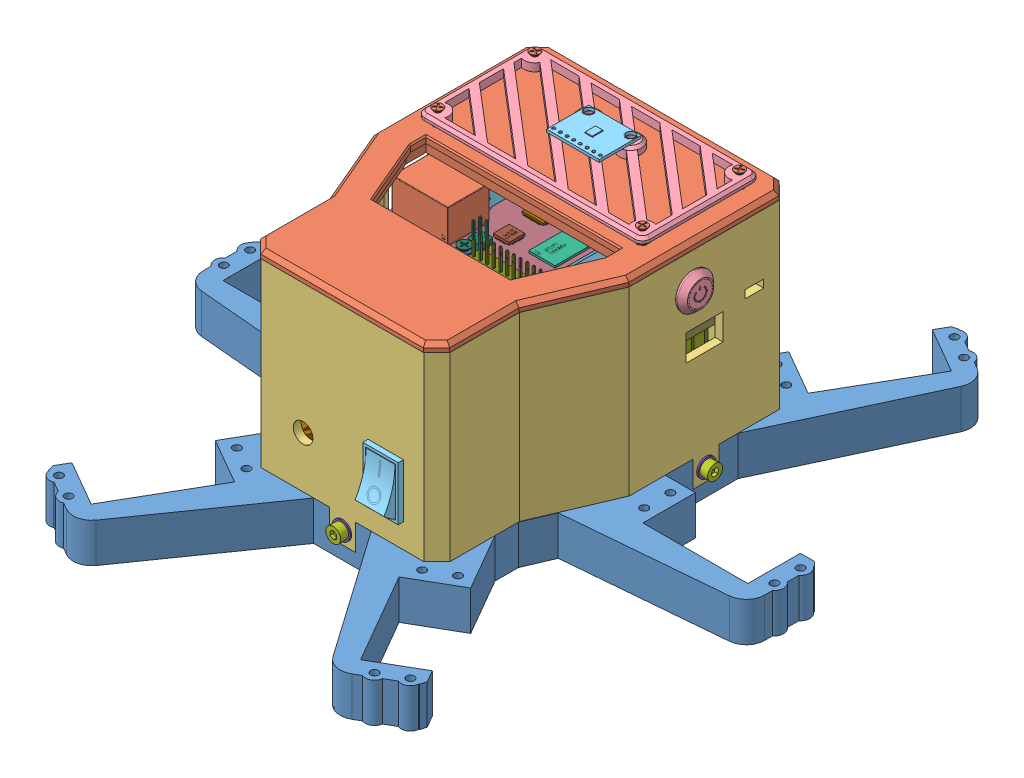
SolidWorks assembly BODY_ASM, configuration Default. Lengths in mm.
Overall size (216.8 93.6 230.48).
146 component instances, 41 part files, 76 mates.
Components (placement in the parent):
- MAIN_FRAME-1: MAIN_FRAME [Default] at origin size (216.8 15 230.48)
- LID-1: LID [Default] at (-25.1298 69 304.4932) x (1 0 0) z (0 1 0) size (97 123 7)
- MID CASE-1: MID CASE [Default] at origin size (97 79 123)
- ON_SWITCH-1: ON_SWITCH [Default] at (33.5 56 5) x (0 0.109318 -0.994007) z (0 -0.994007 -0.109318) size (13.7 18.1 13.7)
- POWER_SWITCH-1: POWER_SWITCH [Default] at (16.5 19.5 76) x (0 -1 0) z (-1 0 0) size (20.5 20.17 13.5)
- M3_HEX_NUT-1: M3_HEX_NUT [Default] at (-35 -5 0) x (0 -0.865861 0.500284) z (0 0.500284 0.865861) size (6.98 2.4 5.5)
- M3_STEEL_HEX_BOLT_16MM-1: M3_STEEL_HEX_BOLT_16MM [Default] at (0 -5 -36.5) x (0.06898 0.997618 0) z (0.997618 -0.06898 0) size (5.68 19 5.68)
- M3_WASHER-1: M3_WASHER [Default] at (-49 -5 0) x (0 -0.533756 -0.845639) z (0 -0.845639 0.533756) size (7 0.5 7)
- M3_HEX_NUT-2: M3_HEX_NUT [Default] at (0 -5 -20.5) x (0.938223 0.346031 0) z (0.346031 -0.938223 0) size (6.98 2.4 5.5)
- M3_HEX_NUT-3: M3_HEX_NUT [Default] at (0 -5 75.1) x (0.997389 -0.072217 0) z (-0.072217 -0.997389 0) size (6.98 2.4 5.5)
- M3_HEX_NUT-4: M3_HEX_NUT [Default] at (32.6 -5 0) x (0 -0.520946 -0.85359) z (0 -0.85359 0.520946) size (6.98 2.4 5.5)
- M3_STEEL_HEX_BOLT_16MM-2: M3_STEEL_HEX_BOLT_16MM [Default] at (-52 -5 0) x (0 -0.536208 -0.844086) z (0 -0.844086 0.536208) size (5.68 19 5.68)
- M3_STEEL_HEX_BOLT_16MM-3: M3_STEEL_HEX_BOLT_16MM [Default] at (52 -5 0) x (0 0.249062 -0.968488) z (0 0.968488 0.249062) size (5.68 19 5.68)
- M3_STEEL_HEX_BOLT_16MM-4: M3_STEEL_HEX_BOLT_16MM [Default] at (0 -5 93.5) x (-0.010084 0.999949 0) z (-0.999949 -0.010084 0) size (5.68 19 5.68)
- M3_WASHER-2: M3_WASHER [Default] at (48.5 -5 0) x (0 -0.753455 -0.657499) z (0 -0.657499 0.753455) size (7 0.5 7)
- M3_WASHER-3: M3_WASHER [Default] at (0 -5 90.5) x (0.583401 0.812184 0) z (-0.812184 0.583401 0) size (7 0.5 7)
- M3_WASHER-4: M3_WASHER [Default] at (0 -5 -33) x (0.7999 0.600134 0) z (-0.600134 0.7999 0) size (7 0.5 7)
- INNER_FRAME_ASM_BRASS-1: INNER_FRAME_ASM_BRASS [Default] at (0 3.6 0) size (89.3 62.14 116.59)
  - power frame R-1: power frame R [Default] at origin size (85 4 113)
  - M2.5_STEEL_HEX_NUT-1: M2.5_STEEL_HEX_NUT [Default] at (39 -1.8 -24.5) x (-0.53176 0 -0.846895) z (0.846895 0 -0.53176) size (6.22 1.8 4.9)
  - M2.5_STEEL_HEX_NUT-2: M2.5_STEEL_HEX_NUT [Default] at (-28.3 -1.8 82.3) x (-0.926596 0 0.376059) z (-0.376059 0 -0.926596) size (6.22 1.8 4.9)
  - M2.5_STEEL_HEX_NUT-3: M2.5_STEEL_HEX_NUT [Default] at (28.3 -1.8 82.3) x (-0.90596 0 -0.423363) z (0.423363 0 -0.90596) size (6.22 1.8 4.9)
  - M2.5_STEEL_HEX_NUT-4: M2.5_STEEL_HEX_NUT [Default] at (-19 -1.8 -24.5) x (0.987479 0 -0.157753) z (0.157753 0 0.987479) size (6.22 1.8 4.9)
  - M2.5_BRASS_SPACER_20MM-1: M2.5_BRASS_SPACER_20MM [Default] at (28.3 16.5 82.3) x (0.147579 0 -0.98905) z (0.98905 0 0.147579) size (5.43 25 4.7)
  - M2.5_BRASS_SPACER_20MM-2: M2.5_BRASS_SPACER_20MM [Default] at (-19 16.5 -24.5) x (0.999419 0 0.034097) z (-0.034097 0 0.999419) size (5.43 25 4.7)
  - M2.5_BRASS_SPACER_20MM-3: M2.5_BRASS_SPACER_20MM [Default] at (-28.3 16.5 82.3) x (0.586169 0 0.810189) z (-0.810189 0 0.586169) size (5.43 25 4.7)
  - M2.5_BRASS_SPACER_20MM-4: M2.5_BRASS_SPACER_20MM [Default] at (39 16.5 -24.5) x (0.00416 0 -0.999991) z (0.999991 0 0.00416) size (5.43 25 4.7)
  - RPi FRAME-1: RPi FRAME [Default] at (0 30.8 0) size (85 4 113)
  - M2.5_STEEL_HEX_NUT-9: M2.5_STEEL_HEX_NUT [Default] at (39 34.8 -24.5) x (0.941663 0 -0.336557) z (0.336557 0 0.941663) size (6.22 1.8 4.9)
  - M2.5_STEEL_HEX_NUT-10: M2.5_STEEL_HEX_NUT [Default] at (28.3 34.8 82.3) x (-0.299428 0 -0.954119) z (0.954119 0 -0.299428) size (6.22 1.8 4.9)
  - M2.5_STEEL_HEX_NUT-11: M2.5_STEEL_HEX_NUT [Default] at (28.3 34.8 45.7) x (-0.609973 0 0.792422) z (-0.792422 0 -0.609973) size (6.22 1.8 4.9)
  - M2.5_STEEL_HEX_NUT-12: M2.5_STEEL_HEX_NUT [Default] at (39 34.8 24.5) x (-0.398443 0 0.917193) z (-0.917193 0 -0.398443) size (6.22 1.8 4.9)
  - M2.5_STEEL_HEX_NUT-13: M2.5_STEEL_HEX_NUT [Default] at (-19 34.8 -24.5) x (-0.889727 0 0.456493) z (-0.456493 0 -0.889727) size (6.22 1.8 4.9)
  - M2.5_STEEL_HEX_NUT-14: M2.5_STEEL_HEX_NUT [Default] at (-19 34.8 24.5) x (-0.550521 0 -0.834821) z (0.834821 0 -0.550521) size (6.22 1.8 4.9)
  - M2.5_STEEL_HEX_NUT-15: M2.5_STEEL_HEX_NUT [Default] at (-28.3 34.8 82.3) x (-0.427939 0 0.903808) z (-0.903808 0 -0.427939) size (6.22 1.8 4.9)
  - M2.5_STEEL_HEX_NUT-16: M2.5_STEEL_HEX_NUT [Default] at (-28.3 34.8 45.7) x (-0.613101 0 -0.790005) z (0.790005 0 -0.613101) size (6.22 1.8 4.9)
  - Raspberry Pi 4 Model B-1: Raspberry Pi 4 Model B [Default] at (0 39.19 0) x (-1 0 0) z (0 0 -1) size (88.99 19.9 58.4)
    - PCB, RPi4ModelB-1: PCB, RPi4ModelB [Default] at origin size (85 1.6 56)
    - Broadcom BCM2711B0 CPU, RPi4ModelB-1: Broadcom BCM2711B0 CPU, RPi4ModelB [Default] at (-13.25 0.8 -4.5) size (15 2.3 15)
    - 2.54 mm DUPONT MALE PIN HEADER, POE, 2X2, RPi4ModelB-1: 2.54 mm DUPONT MALE PIN HEADER, POE, 2X2, RPi4ModelB [Default] at (19 0.8 -18.5) size (5.08 11.3 5.08)
    - 2.54 mm DUPONT MALE PIN HEADER, IO, 2X20, RPi4ModelB-1: 2.54 mm DUPONT MALE PIN HEADER, IO, 2X20, RPi4ModelB [Default] at (-10 0.8 -24.5) size (50.8 11.3 5.08)
    - Camera Connector, RPi4ModelB-1: Camera Connector, RPi4ModelB [Default] at (4 0.8 16.5) x (0 0 -1) z (1 0 0) size (22.4 5.68 5.07)
    - Microphone Plug, RPi4ModelB-1: Microphone Plug, RPi4ModelB [Default] at (11.5 0.8 21.65) size (7.23 7.55 15)
    - Display Connector, RPi4ModelB-1: Display Connector, RPi4ModelB [Default] at (-38.5 0.8 0) x (0 0 1) z (-1 0 0) size (22.4 5.68 5.07)
    - Gigabit Ethernet Port, RPi4ModelB-1: Gigabit Ethernet Port, RPi4ModelB [Default] at (45.5 7.55 -17.75) x (0 0 -1) z (1 0 0) size (16.2 17.24 21.64)
    - Female Micro HDMI Connector, RPi4ModelB-2: Female Micro HDMI Connector, RPi4ModelB [Default] at (-3 0.8 27.3875) size (6.5 3.51 7.5)
    - Female Micro HDMI Connector, RPi4ModelB-3: Female Micro HDMI Connector, RPi4ModelB [Default] at (-16.5 0.8 27.3875) size (6.5 3.51 7.5)
    - Female USB Type C Connector, RPi4ModelB-1: Female USB Type C Connector, RPi4ModelB [Default] at (-31.3 0.8 26.5419) size (8.94 3.96 7.9)
    - 2X USB3.0 PORTS, RPi4ModelB-2: 2X USB3.0 PORTS, RPi4ModelB [Default] at (37.07 0.8 1) size (17.47 19.41 15.68)
    - 91D77 D9WHV 778K, 4 GB LPDDR4 SDRAM, RPi4ModelB-1: 91D77 D9WHV 778K, 4 GB LPDDR4 SDRAM, RPi4ModelB [Default] at (2.25 0.8 -4.5) size (10 0.8 14.5)
    - Cypress CYW43455 Wireless Module Cover, RPi4ModelB-1: Cypress CYW43455 Wireless Module Cover, RPi4ModelB [Default] at (-30.5 0.8 -14.5) size (11 1.6 13)
    - SD Card Slot, RPi4ModelB-1: SD Card Slot, RPi4ModelB [Default] at (-35.3 -0.8 0) x (0 0 -1) z (-1 0 0) size (11.95 1.45 11.4)
    - VIA VL805 PCIe USB 3.0 controller, RPi4ModelB-1: VIA VL805 PCIe USB 3.0 controller, RPi4ModelB [Default] at (17.5 0.8 4) size (8.8 0.8 8.8)
    - 2X USB2.0 PORTS, RPi4ModelB-1: 2X USB2.0 PORTS, RPi4ModelB [Default] at (37.065 0.65 19) size (17.87 19.16 15.33)
    - Broadcom BCM54213PE Gigabit Ethernet Transceiver, RPi4ModelB-1: Broadcom BCM54213PE Gigabit Ethernet Transceiver, RPi4ModelB [Default] at (16.5 0.8 -10) size (6.8 1 6.8)
    - MxL7704 Universal PMIC, RPi4ModelB-1: MxL7704 Universal PMIC, RPi4ModelB [Default] at (-32.5 0.8 16) size (5.4 0.8 5.4)
  - M2.5_STEEL_TRI_BOLT_20MM-1: M2.5_STEEL_TRI_BOLT_20MM [Default] at (39 43.28 -24.5) x (0.010584 0 0.999944) z (0.999944 0 -0.010584) size (4.7 20 4.7)
  - M2.5_STEEL_HEX_NUT-17: M2.5_STEEL_HEX_NUT [Default] at (39 39.98 24.5) x (0.999676 0 0.025448) z (-0.025448 0 0.999676) size (6.22 1.8 4.9)
  - M2.5_STEEL_HEX_NUT-18: M2.5_STEEL_HEX_NUT [Default] at (-28.3 38.2 82.3) x (0.982697 0 -0.185221) z (0.185221 0 0.982697) size (6.22 1.8 4.9)
  - M2.5_STEEL_HEX_NUT-19: M2.5_STEEL_HEX_NUT [Default] at (28.3 38.2 82.3) size (6.22 1.8 4.9)
  - M2.5_STEEL_HEX_NUT-20: M2.5_STEEL_HEX_NUT [Default] at (28.3 38.2 45.7) size (6.22 1.8 4.9)
  - M2.5_STEEL_HEX_NUT-21: M2.5_STEEL_HEX_NUT [Default] at (-28.3 38.2 45.7) size (6.22 1.8 4.9)
  - M2.5_STEEL_HEX_NUT-22: M2.5_STEEL_HEX_NUT [Default] at (-19 39.98 24.5) x (0.99488 0 -0.101065) z (0.101065 0 0.99488) size (6.22 1.8 4.9)
  - M2.5_STEEL_HEX_NUT-23: M2.5_STEEL_HEX_NUT [Default] at (-19 39.98 -24.5) x (0.853732 0 0.520713) z (-0.520713 0 0.853732) size (6.22 1.8 4.9)
  - M2.5_STEEL_HEX_NUT-24: M2.5_STEEL_HEX_NUT [Default] at (39 39.98 -24.5) x (0.977205 0 0.212296) z (-0.212296 0 0.977205) size (6.22 1.8 4.9)
  - M2.5_STEEL_TRI_BOLT_20MM-2: M2.5_STEEL_TRI_BOLT_20MM [Default] at (28.3 41.5 82.3) x (0.000016 0 1) z (1 0 -0.000016) size (4.7 20 4.7)
  - M2.5_STEEL_TRI_BOLT_20MM-3: M2.5_STEEL_TRI_BOLT_20MM [Default] at (-28.3 41.5 82.3) x (0.000016 0 1) z (1 0 -0.000016) size (4.7 20 4.7)
  - M2.5_STEEL_TRI_BOLT_20MM-4: M2.5_STEEL_TRI_BOLT_20MM [Default] at (-19 43.28 -24.5) x (0.000016 0 1) z (1 0 -0.000016) size (4.7 20 4.7)
  - SERVO_2040-1: SERVO_2040 [Default] at (0 36.6 64) x (-1 0 0) z (0 0 -1) size (63.5 10.6 42)
  - M2.5_NYLON_BOLT-1: M2.5_NYLON_BOLT [Default] at (-28.3 41.5 45.7) x (0.149804 0 0.988716) z (0.988716 0 -0.149804) size (4.7 15 4.7)
  - M2.5_NYLON_BOLT-2: M2.5_NYLON_BOLT [Default] at (39 43.28 24.5) x (0.149804 0 0.988716) z (0.988716 0 -0.149804) size (4.7 15 4.7)
  - M2.5_NYLON_BOLT-3: M2.5_NYLON_BOLT [Default] at (28.3 41.5 45.7) x (0.149804 0 0.988716) z (0.988716 0 -0.149804) size (4.7 15 4.7)
  - M2.5_NYLON_BOLT-4: M2.5_NYLON_BOLT [Default] at (-19 43.28 24.5) x (0.05042 0 -0.998728) z (-0.998728 0 -0.05042) size (4.7 15 4.7)
  - M2.5_STEEL_HEX_NUT-25: M2.5_STEEL_HEX_NUT [Default] at (28.3 29 45.7) size (6.22 1.8 4.9)
  - M2.5_STEEL_HEX_NUT-26: M2.5_STEEL_HEX_NUT [Default] at (-28.3 29 45.7) x (0.960779 0 0.277315) z (-0.277315 0 0.960779) size (6.22 1.8 4.9)
  - M2.5_STEEL_HEX_NUT-27: M2.5_STEEL_HEX_NUT [Default] at (-19 29 24.5) x (0.999926 0 0.01217) z (-0.01217 0 0.999926) size (6.22 1.8 4.9)
  - M2.5_STEEL_HEX_NUT-28: M2.5_STEEL_HEX_NUT [Default] at (39 29 24.5) x (0.999999 0 -0.001638) z (0.001638 0 0.999999) size (6.22 1.8 4.9)
  - 7V_BUCK-1: 7V_BUCK [Default] at (13.575 6 12.675) x (0 0 1) z (-1 0 0) size (65.3 21.55 50.1)
  - 3.3V_RELAY-1: 3.3V_RELAY [Default] at (-21.55 5.2 16.3) x (0 0 1) z (-1 0 0) size (70 18 17)
  - M2.5_NYLON_HEX_NUT-1: M2.5_NYLON_HEX_NUT [Default] at (0.65 -2 41.35) size (5.66 2 4.9)
  - M2.5_NYLON_HEX_NUT-2: M2.5_NYLON_HEX_NUT [Default] at (26.5 4 -16) size (5.66 2 4.9)
  - M2.5_NYLON_HEX_NUT-3: M2.5_NYLON_HEX_NUT [Default] at (0.65 4 41.35) size (5.66 2 4.9)
  - M2.5_NYLON_HEX_NUT-4: M2.5_NYLON_HEX_NUT [Default] at (26.5 -2 41.35) size (5.66 2 4.9)
  - M2.5_NYLON_HEX_NUT-5: M2.5_NYLON_HEX_NUT [Default] at (26.5 4 41.35) size (5.66 2 4.9)
  - M2.5_NYLON_HEX_NUT-6: M2.5_NYLON_HEX_NUT [Default] at (0.65 4 -16) size (5.66 2 4.9)
  - M2.5_NYLON_HEX_NUT-7: M2.5_NYLON_HEX_NUT [Default] at (0.65 -2 -16) size (5.66 2 4.9)
  - M2.5_NYLON_HEX_NUT-8: M2.5_NYLON_HEX_NUT [Default] at (26.5 -2 -16) size (5.66 2 4.9)
  - M2_NYLON_HEX_NUT-1: M2_NYLON_HEX_NUT [Default] at (-27.75 4 -16) size (4.39 1.2 3.8)
  - M2_NYLON_HEX_NUT-2: M2_NYLON_HEX_NUT [Default] at (-27.75 -1.2 48.6) x (0.996977 0 0.0777) z (-0.0777 0 0.996977) size (4.39 1.2 3.8)
  - M2_NYLON_HEX_NUT-3: M2_NYLON_HEX_NUT [Default] at (-15.35 4 -16) size (4.39 1.2 3.8)
  - M2_NYLON_HEX_NUT-5: M2_NYLON_HEX_NUT [Default] at (-15.35 -1.2 48.6) size (4.39 1.2 3.8)
  - M2_NYLON_HEX_NUT-6: M2_NYLON_HEX_NUT [Default] at (-15.35 -1.2 -16) x (-0.796408 0 -0.604759) z (0.604759 0 -0.796408) size (4.39 1.2 3.8)
  - M2_NYLON_HEX_NUT-8: M2_NYLON_HEX_NUT [Default] at (-27.75 -1.2 -16) x (-0.852858 0 0.522143) z (-0.522143 0 -0.852858) size (4.39 1.2 3.8)
  - M2_NYLON_HEX_NUT-9: M2_NYLON_HEX_NUT [Default] at (-27.75 4 48.6) size (4.39 1.2 3.8)
  - M2_NYLON_HEX_NUT-10: M2_NYLON_HEX_NUT [Default] at (-15.35 4 48.6) size (4.39 1.2 3.8)
  - M2.5_STEEL_HEX_NUT-29: M2.5_STEEL_HEX_NUT [Default] at (-28.3 29 82.3) x (-0.398443 0 0.917193) z (-0.917193 0 -0.398443) size (6.22 1.8 4.9)
  - M2.5_STEEL_HEX_NUT-30: M2.5_STEEL_HEX_NUT [Default] at (-19 29 -24.5) x (-0.398443 0 0.917193) z (-0.917193 0 -0.398443) size (6.22 1.8 4.9)
  - M2.5_STEEL_HEX_NUT-31: M2.5_STEEL_HEX_NUT [Default] at (28.3 29 82.3) x (-0.187174 0 0.982327) z (-0.982327 0 -0.187174) size (6.22 1.8 4.9)
  - M2.5_STEEL_HEX_NUT-32: M2.5_STEEL_HEX_NUT [Default] at (39 29 -24.5) x (-0.432758 0 0.90151) z (-0.90151 0 -0.432758) size (6.22 1.8 4.9)
  - M2.5_NYLON_BOLT-5: M2.5_NYLON_BOLT [Default] at (26.5 9.05 41.35) x (0.298465 0 -0.954421) z (-0.954421 0 -0.298465) size (4.7 15 4.7)
  - M2.5_NYLON_BOLT-6: M2.5_NYLON_BOLT [Default] at (0.65 9.05 -16) x (0.311969 0 -0.950092) z (-0.950092 0 -0.311969) size (4.7 15 4.7)
  - M2.5_NYLON_BOLT-7: M2.5_NYLON_BOLT [Default] at (26.5 9.05 -16) x (0.298465 0 -0.954421) z (-0.954421 0 -0.298465) size (4.7 15 4.7)
  - M2.5_NYLON_BOLT-8: M2.5_NYLON_BOLT [Default] at (0.65 9.05 41.35) x (0.298465 0 -0.954421) z (-0.954421 0 -0.298465) size (4.7 15 4.7)
  - M2_NYLON_BOLT-1: M2_NYLON_BOLT [Default] at (-27.75 7.8 48.6) x (-0.556663 0 -0.830738) z (-0.830738 0 0.556663) size (3.8 10 3.8)
  - M2_NYLON_BOLT-2: M2_NYLON_BOLT [Default] at (-15.35 7.8 48.6) x (-0.518121 0 -0.855307) z (-0.855307 0 0.518121) size (3.8 10 3.8)
  - M2_NYLON_BOLT-3: M2_NYLON_BOLT [Default] at (-27.75 7.8 -16) x (-0.556663 0 -0.830738) z (-0.830738 0 0.556663) size (3.8 10 3.8)
  - M2_NYLON_BOLT-4: M2_NYLON_BOLT [Default] at (-15.35 7.8 -16) x (-0.556663 0 -0.830738) z (-0.830738 0 0.556663) size (3.8 10 3.8)
  - 5v_buck-1: 5v_buck [Default] at (19 31.6 -14) x (1 0 0) z (0 0 -1) size (33 7.8 28.5)
  - M2_NYLON_BOLT-5: M2_NYLON_BOLT [Default] at (32.95 35.9 -15.7) x (0.89104 0 -0.453925) z (-0.453925 0 -0.89104) size (3.8 10 3.8)
  - M2_NYLON_BOLT-6: M2_NYLON_BOLT [Default] at (5.05 35.9 -2.5) x (0.891706 0 -0.452615) z (-0.452615 0 -0.891706) size (3.8 10 3.8)
  - M2_NYLON_BOLT-7: M2_NYLON_BOLT [Default] at (5.05 35.9 -15.7) x (0.896031 0 -0.443992) z (-0.443992 0 -0.896031) size (3.8 10 3.8)
  - M2_NYLON_BOLT-8: M2_NYLON_BOLT [Default] at (32.95 35.9 -2.5) x (0.891706 0 -0.452615) z (-0.452615 0 -0.891706) size (3.8 10 3.8)
  - M2_NYLON_HEX_NUT-11: M2_NYLON_HEX_NUT [Default] at (32.95 31.6 -2.5) size (4.39 1.2 3.8)
  - M2_NYLON_HEX_NUT-12: M2_NYLON_HEX_NUT [Default] at (32.95 31.6 -15.7) size (4.39 1.2 3.8)
  - M2_NYLON_HEX_NUT-13: M2_NYLON_HEX_NUT [Default] at (5.05 31.6 -2.5) size (4.39 1.2 3.8)
  - M2_NYLON_HEX_NUT-14: M2_NYLON_HEX_NUT [Default] at (5.05 31.6 -15.7) size (4.39 1.2 3.8)
  - M2_NYLON_HEX_NUT-15: M2_NYLON_HEX_NUT [Default] at (32.95 28.9 -15.7) size (4.39 1.2 3.8)
  - M2_NYLON_HEX_NUT-16: M2_NYLON_HEX_NUT [Default] at (5.05 28.9 -15.7) size (4.39 1.2 3.8)
  - M2_NYLON_HEX_NUT-17: M2_NYLON_HEX_NUT [Default] at (32.95 28.9 -2.5) size (4.39 1.2 3.8)
  - M2_NYLON_HEX_NUT-18: M2_NYLON_HEX_NUT [Default] at (5.05 28.9 -2.5) size (4.39 1.2 3.8)
  - M2.5_STEEL_HEX_NUT-33: M2.5_STEEL_HEX_NUT [Default] at (-19 36.6 -24.5) x (-0.398443 0 0.917193) z (-0.917193 0 -0.398443) size (6.22 1.8 4.9)
  - M2.5_STEEL_HEX_NUT-34: M2.5_STEEL_HEX_NUT [Default] at (39 36.6 24.5) x (-0.398443 0 0.917193) z (-0.917193 0 -0.398443) size (6.22 1.8 4.9)
  - M2.5_STEEL_HEX_NUT-35: M2.5_STEEL_HEX_NUT [Default] at (-19 36.6 24.5) x (-0.398443 0 0.917193) z (-0.917193 0 -0.398443) size (6.22 1.8 4.9)
  - M2.5_STEEL_HEX_NUT-36: M2.5_STEEL_HEX_NUT [Default] at (39 36.6 -24.5) x (-0.398443 0 0.917193) z (-0.917193 0 -0.398443) size (6.22 1.8 4.9)
  - M2.5_STEEL_HEX_NUT-37: M2.5_STEEL_HEX_NUT [Default] at (39 -3.6 -24.5) x (-0.586704 0 -0.809801) z (0.809801 0 -0.586704) size (6.22 1.8 4.9)
  - M2.5_STEEL_HEX_NUT-38: M2.5_STEEL_HEX_NUT [Default] at (28.3 -3.6 82.3) x (-0.456254 0 -0.889849) z (0.889849 0 -0.456254) size (6.22 1.8 4.9)
  - M2.5_STEEL_HEX_NUT-39: M2.5_STEEL_HEX_NUT [Default] at (-19 -3.6 -24.5) x (0.101594 0 -0.994826) z (0.994826 0 0.101594) size (6.22 1.8 4.9)
  - M2.5_STEEL_HEX_NUT-40: M2.5_STEEL_HEX_NUT [Default] at (-28.3 -3.6 82.3) x (-0.455411 0 -0.890281) z (0.890281 0 -0.455411) size (6.22 1.8 4.9)
- M2.5_STEEL_TRI_BOLT_20MM-1: M2.5_STEEL_TRI_BOLT_20MM [Default] at (-19 -8.65 -24.5) x (0.913498 0 -0.406843) z (0.406843 0 0.913498) size (4.7 20 4.7)
- M2.5_STEEL_TRI_BOLT_20MM-2: M2.5_STEEL_TRI_BOLT_20MM [Default] at (28.3 -8.65 82.3) x (-0.766419 0 0.642341) z (-0.642341 0 -0.766419) size (4.7 20 4.7)
- M2.5_STEEL_TRI_BOLT_20MM-3: M2.5_STEEL_TRI_BOLT_20MM [Default] at (-28.3 -8.65 82.3) x (-0.697743 0 -0.716349) z (0.716349 0 -0.697743) size (4.7 20 4.7)
- M2.5_STEEL_TRI_BOLT_20MM-4: M2.5_STEEL_TRI_BOLT_20MM [Default] at (39 -8.65 -24.5) x (0.943102 0 -0.332503) z (0.332503 0 0.943102) size (4.7 20 4.7)
- M2_NYLON_BOLT-1: M2_NYLON_BOLT [Default] at (38.915 77.3 -22.415) x (0.869496 0 -0.49394) z (-0.49394 0 -0.869496) size (3.8 10 3.8)
- M2_NYLON_HEX_NUT-1: M2_NYLON_HEX_NUT [Default] at (-39.085 67.8 14.585) size (4.39 1.2 3.8)
- M2_NYLON_HEX_NUT-2: M2_NYLON_HEX_NUT [Default] at (38.915 67.8 14.585) size (4.39 1.2 3.8)
- M2_NYLON_HEX_NUT-3: M2_NYLON_HEX_NUT [Default] at (-39.085 67.8 -22.415) size (4.39 1.2 3.8)
- M2_NYLON_HEX_NUT-4: M2_NYLON_HEX_NUT [Default] at (38.915 67.8 -22.415) size (4.39 1.2 3.8)
- M2_NYLON_BOLT-2: M2_NYLON_BOLT [Default] at (-39.085 77.3 -22.415) x (0.562561 0 -0.826756) z (-0.826756 0 -0.562561) size (3.8 10 3.8)
- M2_NYLON_BOLT-3: M2_NYLON_BOLT [Default] at (38.915 77.3 14.585) x (0.001977 0 -0.999998) z (-0.999998 0 -0.001977) size (3.8 10 3.8)
- M2_NYLON_BOLT-4: M2_NYLON_BOLT [Default] at (-39.085 77.3 14.585) x (0.810874 0 -0.585221) z (-0.585221 0 -0.810874) size (3.8 10 3.8)
- M2_NYLON_HEX_NUT-5: M2_NYLON_HEX_NUT [Default] at (-39.085 72 -22.415) x (0.987617 0 -0.156887) z (0.156887 0 0.987617) size (4.39 1.2 3.8)
- M2_NYLON_HEX_NUT-6: M2_NYLON_HEX_NUT [Default] at (-39.085 72 14.585) x (0.982983 0 0.183699) z (-0.183699 0 0.982983) size (4.39 1.2 3.8)
- M2_NYLON_HEX_NUT-7: M2_NYLON_HEX_NUT [Default] at (38.915 72 14.585) x (0.858157 0 0.513388) z (-0.513388 0 0.858157) size (4.39 1.2 3.8)
- M2_NYLON_HEX_NUT-8: M2_NYLON_HEX_NUT [Default] at (38.915 72 -22.415) x (0.965887 0 0.258962) z (-0.258962 0 0.965887) size (4.39 1.2 3.8)
- MPU6050_STAND-3: MPU6050_STAND [Default] at (-0.085 73.2 -3.915) x (-1 0 0) z (0 0 -1) size (86 4 45)
- Gyroscope sensor-1: Gyroscope sensor [Default] at (-0.085 77.2 -5.915) x (0 0 -1) z (1 0 0) size (16 1.4 20)
Mates (geometry in assembly coordinates):
- Coincident1: coordinate: point of MAIN_FRAME-1
- Concentric13: concentric aligned: cylinder of MAIN_FRAME-1 through (107 -5 0) axis (-1 0 0) radius 2; cylinder of MID CASE-1 through (48.5 -5 0) axis (-1 0 0) radius 1.75
- Concentric14: concentric aligned: cylinder of MAIN_FRAME-1 through (0 -5 141.7159) axis (0 0 -1) radius 2; cylinder of MID CASE-1 through (0 -5 90) axis (0 0 -1) radius 1.75
- Distance1: distance = 0.065 mm anti-aligned: plane of LID-1 through (-42.4045 65 -30.065) normal (0 0 -1); plane of MID CASE-1 through (-45.5 69 -30) normal (0 0 1)
- Distance2: distance = 0.065 mm anti-aligned: plane of LID-1 through (45.565 65 -26.7345) normal (1 0 0); plane of MID CASE-1 through (45.5 69 -30) normal (-1 0 0)
- Coincident14: coincident anti-aligned: plane of LID-1 through (-25.1298 69 304.4932) normal (0 -1 0); plane of MID CASE-1 through (0 69 0) normal (0 1 0)
- Concentric15: concentric anti-aligned: cylinder of MID CASE-1 through (-48.501 56 5) axis (1 0 0) radius 6; cylinder of ON_SWITCH-1 through (49.5 56 5) axis (-1 0 0) radius 5.8
- Distance3: distance = 1 mm anti-aligned: plane of MID CASE-1 through (48.5 69 -33) normal (1 0 0); plane of ON_SWITCH-1 through (49.5 56 5) normal (-1 0 0)
- Coincident20: coincident anti-aligned: plane of MID CASE-1 through (10 10 -33.001) normal (1 0 0); plane of POWER_SWITCH-1 through (10 29 90) normal (-1 0 0)
- Coincident21: coincident anti-aligned: plane of MID CASE-1 through (23 29 -33.001) normal (0 -1 0); plane of POWER_SWITCH-1 through (10 29 90) normal (0 1 0)
- Coincident22: coincident anti-aligned: plane of MID CASE-1 through (36 69 90) normal (0 0 1); plane of POWER_SWITCH-1 through (16.5 19.5 90) normal (0 0 -1)
- Concentric16: concentric aligned: cylinder of MID CASE-1 through (48.5 -5 0) axis (-1 0 0) radius 1.75; cylinder of M3_WASHER-1 through (-48.5 -5 0) axis (-1 0 0) radius 1.6
- Coincident23: coincident anti-aligned: plane of MID CASE-1 through (-48.5 69 29.2246) normal (-1 0 0); plane of M3_WASHER-1 through (-48.5 -5 0) normal (1 0 0)
- Coincident25: coincident anti-aligned: plane of MID CASE-1 through (48.5 69 -33) normal (1 0 0); plane of M3_WASHER-2 through (48.5 -5 0) normal (-1 0 0)
- Concentric18: concentric aligned: cylinder of MID CASE-1 through (48.5 -5 0) axis (-1 0 0) radius 1.75; cylinder of M3_WASHER-2 through (49 -5 0) axis (-1 0 0) radius 1.6
- Coincident26: coincident anti-aligned: plane of MID CASE-1 through (-48.5 69 -33) normal (0 0 -1); plane of M3_WASHER-4 through (0 -5 -33) normal (0 0 1)
- Concentric19: concentric anti-aligned: cylinder of MID CASE-1 through (0 -5 90) axis (0 0 -1) radius 1.75; cylinder of M3_WASHER-4 through (0 -5 -33.5) axis (0 0 1) radius 1.6
- Coincident27: coincident anti-aligned: plane of MID CASE-1 through (36 69 90) normal (0 0 1); plane of M3_WASHER-3 through (0 -5 90) normal (0 0 -1)
- Concentric20: concentric anti-aligned: cylinder of MID CASE-1 through (0 -5 90) axis (0 0 -1) radius 1.75; cylinder of M3_WASHER-3 through (0 -5 90) axis (0 0 1) radius 1.6
- Coincident31: coincident anti-aligned: plane of MAIN_FRAME-1 through (35 -15 -20.5) normal (-1 0 0); plane of M3_HEX_NUT-4 through (35 -5 0) normal (1 0 0)
- Concentric24: concentric aligned: cylinder of MAIN_FRAME-1 through (107 -5 0) axis (-1 0 0) radius 2; cylinder of M3_HEX_NUT-4 through (35 -5 0) axis (-1 0 0) radius 1.5
- Coincident33: coincident anti-aligned: plane of MAIN_FRAME-1 through (-35 -15 -20.5) normal (1 0 0); plane of M3_HEX_NUT-1 through (-35 -5 0) normal (-1 0 0)
- Concentric25: concentric aligned: cylinder of MAIN_FRAME-1 through (107 -5 0) axis (-1 0 0) radius 2; cylinder of M3_HEX_NUT-1 through (-32.6 -5 0) axis (-1 0 0) radius 1.5
- Coincident34: coincident anti-aligned: plane of MAIN_FRAME-1 through (0 -15 -20.5) normal (0 0 1); plane of M3_HEX_NUT-2 through (0 -5 -20.5) normal (0 0 -1)
- Concentric26: concentric aligned: cylinder of MAIN_FRAME-1 through (0 -5 141.7159) axis (0 0 -1) radius 2; cylinder of M3_HEX_NUT-2 through (0 -5 -18.1) axis (0 0 -1) radius 1.5
- Coincident35: coincident anti-aligned: plane of MAIN_FRAME-1 through (0 -15 77.5) normal (0 0 -1); plane of M3_HEX_NUT-3 through (0 -5 77.5) normal (0 0 1)
- Concentric27: concentric aligned: cylinder of MAIN_FRAME-1 through (0 -5 141.7159) axis (0 0 -1) radius 2; cylinder of M3_HEX_NUT-3 through (0 -5 77.5) axis (0 0 -1) radius 1.5
- Concentric28: concentric aligned: cylinder of MID CASE-1 through (0 -5 90) axis (0 0 -1) radius 1.75; cylinder of M3_STEEL_HEX_BOLT_16MM-1 through (0 -5 -17.5) axis (0 0 -1) radius 1.5
- Coincident36: coincident anti-aligned: plane of M3_STEEL_HEX_BOLT_16MM-1 through (0 -5 -33.5) normal (0 0 1); plane of M3_WASHER-4 through (0 -5 -33.5) normal (0 0 -1)
- Concentric29: concentric aligned: cylinder of MID CASE-1 through (48.5 -5 0) axis (-1 0 0) radius 1.75; cylinder of M3_STEEL_HEX_BOLT_16MM-2 through (-33 -5 0) axis (-1 0 0) radius 1.5
- Coincident37: coincident anti-aligned: plane of M3_WASHER-1 through (-49 -5 0) normal (-1 0 0); plane of M3_STEEL_HEX_BOLT_16MM-2 through (-49 -5 0) normal (1 0 0)
- Coincident38: coincident anti-aligned: plane of M3_STEEL_HEX_BOLT_16MM-3 through (49 -5 0) normal (-1 0 0); plane of M3_WASHER-2 through (49 -5 0) normal (1 0 0)
- Concentric30: concentric anti-aligned: cylinder of MID CASE-1 through (48.5 -5 0) axis (-1 0 0) radius 1.75; cylinder of M3_STEEL_HEX_BOLT_16MM-3 through (33 -5 0) axis (1 0 0) radius 1.5
- Coincident39: coincident anti-aligned: plane of M3_STEEL_HEX_BOLT_16MM-4 through (0 -5 90.5) normal (0 0 -1); plane of M3_WASHER-3 through (0 -5 90.5) normal (0 0 1)
- Concentric31: concentric anti-aligned: cylinder of MID CASE-1 through (0 -5 90) axis (0 0 -1) radius 1.75; cylinder of M3_STEEL_HEX_BOLT_16MM-4 through (0 -5 74.5) axis (0 0 1) radius 1.5
- Concentric32: concentric anti-aligned: cylinder of MAIN_FRAME-1 through (-19 -15 -24.5) axis (0 1 0) radius 1.4; cylinder of INNER_FRAME_ASM_BRASS-1/M2.5_STEEL_HEX_NUT-4 through (-19 3.6 -24.5) axis (0 -1 0) radius 1.25
- Concentric33: concentric anti-aligned: cylinder of MAIN_FRAME-1 through (28.3 -15 82.3) axis (0 1 0) radius 1.4; cylinder of INNER_FRAME_ASM_BRASS-1/M2.5_STEEL_HEX_NUT-3 through (28.3 3.6 82.3) axis (0 -1 0) radius 1.25
- Concentric34: concentric aligned: cylinder of INNER_FRAME_ASM_BRASS-1/M2.5_BRASS_SPACER_20MM-4 through (39 14.6 -24.5) axis (0 -1 0) radius 1.25; cylinder of M2.5_STEEL_TRI_BOLT_20MM-4 through (39 11.35 -24.5) axis (0 -1 0) radius 1.25
- Concentric36: concentric aligned: cylinder of INNER_FRAME_ASM_BRASS-1/M2.5_BRASS_SPACER_20MM-1 through (28.3 14.6 82.3) axis (0 -1 0) radius 1.25; cylinder of M2.5_STEEL_TRI_BOLT_20MM-2 through (28.3 11.35 82.3) axis (0 -1 0) radius 1.25
- Concentric38: concentric aligned: cylinder of INNER_FRAME_ASM_BRASS-1/M2.5_BRASS_SPACER_20MM-2 through (-19 14.6 -24.5) axis (0 -1 0) radius 1.25; cylinder of M2.5_STEEL_TRI_BOLT_20MM-1 through (-19 11.35 -24.5) axis (0 -1 0) radius 1.25
- Concentric40: concentric aligned: cylinder of INNER_FRAME_ASM_BRASS-1/M2.5_BRASS_SPACER_20MM-3 through (-28.3 14.6 82.3) axis (0 -1 0) radius 1.25; cylinder of M2.5_STEEL_TRI_BOLT_20MM-3 through (-28.3 11.35 82.3) axis (0 -1 0) radius 1.25
- Coincident41: coincident aligned: cone of MAIN_FRAME-1 through (39 -9 -24.5) axis (0 1 0); cone of M2.5_STEEL_TRI_BOLT_20MM-4 through (39 -7.15 -24.5) axis (0 1 0)
- Coincident42: coincident aligned: cone of MAIN_FRAME-1 through (-19 -9 -24.5) axis (0 1 0); cone of M2.5_STEEL_TRI_BOLT_20MM-1 through (-19 -7.15 -24.5) axis (0 1 0)
- Coincident43: coincident aligned: cone of MAIN_FRAME-1 through (-28.3 -9 82.3) axis (0 1 0); cone of M2.5_STEEL_TRI_BOLT_20MM-3 through (-28.3 -7.15 82.3) axis (0 1 0)
- Coincident44: coincident aligned: cone of MAIN_FRAME-1 through (28.3 -9 82.3) axis (0 1 0); cone of M2.5_STEEL_TRI_BOLT_20MM-2 through (28.3 -7.15 82.3) axis (0 1 0)
- Concentric41: concentric anti-aligned: cylinder of LID-1 through (38.915 64.999 14.585) axis (0 1 0) radius 1.25; cylinder of M2_NYLON_HEX_NUT-2 through (38.915 69 14.585) axis (0 -1 0) radius 1
- Concentric42: concentric anti-aligned: cylinder of LID-1 through (38.915 64.999 -22.415) axis (0 1 0) radius 1.25; cylinder of M2_NYLON_HEX_NUT-4 through (38.915 69 -22.415) axis (0 -1 0) radius 1
- Concentric43: concentric anti-aligned: cylinder of LID-1 through (-39.085 64.999 14.585) axis (0 1 0) radius 1.25; cylinder of M2_NYLON_HEX_NUT-1 through (-39.085 69 14.585) axis (0 -1 0) radius 1
- Concentric44: concentric anti-aligned: cylinder of LID-1 through (-39.085 64.999 -22.415) axis (0 1 0) radius 1.25; cylinder of M2_NYLON_HEX_NUT-3 through (-39.085 69 -22.415) axis (0 -1 0) radius 1
- Coincident48: coincident anti-aligned: plane of LID-1 through (-25.1298 69 304.4932) normal (0 -1 0); plane of M2_NYLON_HEX_NUT-3 through (-39.085 69 -22.415) normal (0 1 0)
- Coincident49: coincident anti-aligned: plane of LID-1 through (-25.1298 69 304.4932) normal (0 -1 0); plane of M2_NYLON_HEX_NUT-4 through (38.915 69 -22.415) normal (0 1 0)
- Coincident50: coincident anti-aligned: plane of LID-1 through (-25.1298 69 304.4932) normal (0 -1 0); plane of M2_NYLON_HEX_NUT-2 through (38.915 69 14.585) normal (0 1 0)
- Coincident51: coincident anti-aligned: plane of LID-1 through (-25.1298 69 304.4932) normal (0 -1 0); plane of M2_NYLON_HEX_NUT-1 through (-39.085 69 14.585) normal (0 1 0)
- Concentric51: concentric anti-aligned: cylinder of LID-1 through (38.915 64.999 -22.415) axis (0 1 0) radius 1.25; cylinder of M2_NYLON_HEX_NUT-8 through (38.915 73.2 -22.415) axis (0 -1 0) radius 1
- Concentric52: concentric anti-aligned: cylinder of LID-1 through (38.915 64.999 14.585) axis (0 1 0) radius 1.25; cylinder of M2_NYLON_HEX_NUT-7 through (38.915 73.2 14.585) axis (0 -1 0) radius 1
- Concentric53: concentric anti-aligned: cylinder of LID-1 through (-39.085 64.999 14.585) axis (0 1 0) radius 1.25; cylinder of M2_NYLON_HEX_NUT-6 through (-39.085 73.2 14.585) axis (0 -1 0) radius 1
- Concentric54: concentric anti-aligned: cylinder of LID-1 through (-39.085 64.999 -22.415) axis (0 1 0) radius 1.25; cylinder of M2_NYLON_HEX_NUT-5 through (-39.085 73.2 -22.415) axis (0 -1 0) radius 1
- Coincident56: coincident anti-aligned: plane of LID-1 through (-25.1298 72 304.4932) normal (0 1 0); plane of M2_NYLON_HEX_NUT-8 through (38.915 72 -22.415) normal (0 -1 0)
- Coincident57: coincident anti-aligned: plane of LID-1 through (-25.1298 72 304.4932) normal (0 1 0); plane of M2_NYLON_HEX_NUT-7 through (38.915 72 14.585) normal (0 -1 0)
- Coincident58: coincident anti-aligned: plane of LID-1 through (-25.1298 72 304.4932) normal (0 1 0); plane of M2_NYLON_HEX_NUT-5 through (-39.085 72 -22.415) normal (0 -1 0)
- Coincident59: coincident anti-aligned: plane of LID-1 through (-25.1298 72 304.4932) normal (0 1 0); plane of M2_NYLON_HEX_NUT-6 through (-39.085 72 14.585) normal (0 -1 0)
- Concentric55: concentric aligned: cylinder of LID-1 through (38.915 64.999 -22.415) axis (0 1 0) radius 1.25; cylinder of M2_NYLON_BOLT-1 through (38.915 67.3 -22.415) axis (0 1 0) radius 1
- Concentric56: concentric anti-aligned: cylinder of M2_NYLON_BOLT-3 through (38.915 67.3 14.585) axis (0 1 0) radius 1; cylinder of M2_NYLON_HEX_NUT-7 through (38.915 73.2 14.585) axis (0 -1 0) radius 1
- Concentric57: concentric anti-aligned: cylinder of M2_NYLON_BOLT-4 through (-39.085 67.3 14.585) axis (0 1 0) radius 1; cylinder of M2_NYLON_HEX_NUT-6 through (-39.085 73.2 14.585) axis (0 -1 0) radius 1
- Concentric58: concentric anti-aligned: cylinder of M2_NYLON_BOLT-2 through (-39.085 67.3 -22.415) axis (0 1 0) radius 1; cylinder of M2_NYLON_HEX_NUT-5 through (-39.085 73.2 -22.415) axis (0 -1 0) radius 1
- Coincident67: coincident anti-aligned: plane of MAIN_FRAME-1 through (34 0 55.6123) normal (0 1 0); plane of INNER_FRAME_ASM_BRASS-1/M2.5_STEEL_HEX_NUT-39 through (-19 0 -24.5) normal (0 -1 0)
- Concentric59: concentric anti-aligned: cylinder of M2_NYLON_BOLT-2 through (-39.085 67.3 -22.415) axis (0 1 0) radius 1; cylinder of MPU6050_STAND-3 through (-39.085 76.2 -22.415) axis (0 -1 0) radius 1.25
- Concentric60: concentric anti-aligned: cylinder of M2_NYLON_BOLT-3 through (38.915 67.3 14.585) axis (0 1 0) radius 1; cylinder of MPU6050_STAND-3 through (38.915 76.2 14.585) axis (0 -1 0) radius 1.25
- Coincident68: coincident anti-aligned: plane of M2_NYLON_HEX_NUT-8 through (38.915 73.2 -22.415) normal (0 1 0); plane of MPU6050_STAND-3 through (-0.085 73.2 -3.915) normal (0 -1 0)
- Coincident69: coincident anti-aligned: circle of M2_NYLON_BOLT-1; plane of MPU6050_STAND-3 through (-0.085 76.2 -3.915) normal (0 1 0)
- Coincident70: coincident anti-aligned: circle of M2_NYLON_BOLT-3; plane of MPU6050_STAND-3 through (-0.085 76.2 -3.915) normal (0 1 0)
- Coincident71: coincident anti-aligned: circle of M2_NYLON_BOLT-4; plane of MPU6050_STAND-3 through (-0.085 76.2 -3.915) normal (0 1 0)
- Coincident72: coincident anti-aligned: circle of M2_NYLON_BOLT-2; plane of MPU6050_STAND-3 through (-0.085 76.2 -3.915) normal (0 1 0)
- Concentric61: concentric anti-aligned: cylinder of MPU6050_STAND-3 through (7.915 73.2 -11.915) axis (0 1 0) radius 1.5; cylinder of Gyroscope sensor-1 through (7.915 78.3 -11.915) axis (0 -1 0) radius 1.6
- Concentric62: concentric anti-aligned: cylinder of MPU6050_STAND-3 through (-8.085 73.2 -11.915) axis (0 1 0) radius 1.5; cylinder of Gyroscope sensor-1 through (-8.085 78.3 -11.915) axis (0 -1 0) radius 1.6
- Coincident73: coincident anti-aligned: plane of MPU6050_STAND-3 through (-8.085 77.2 -11.915) normal (0 1 0); plane of Gyroscope sensor-1 through (-0.085 77.2 -5.915) normal (0 -1 0)
